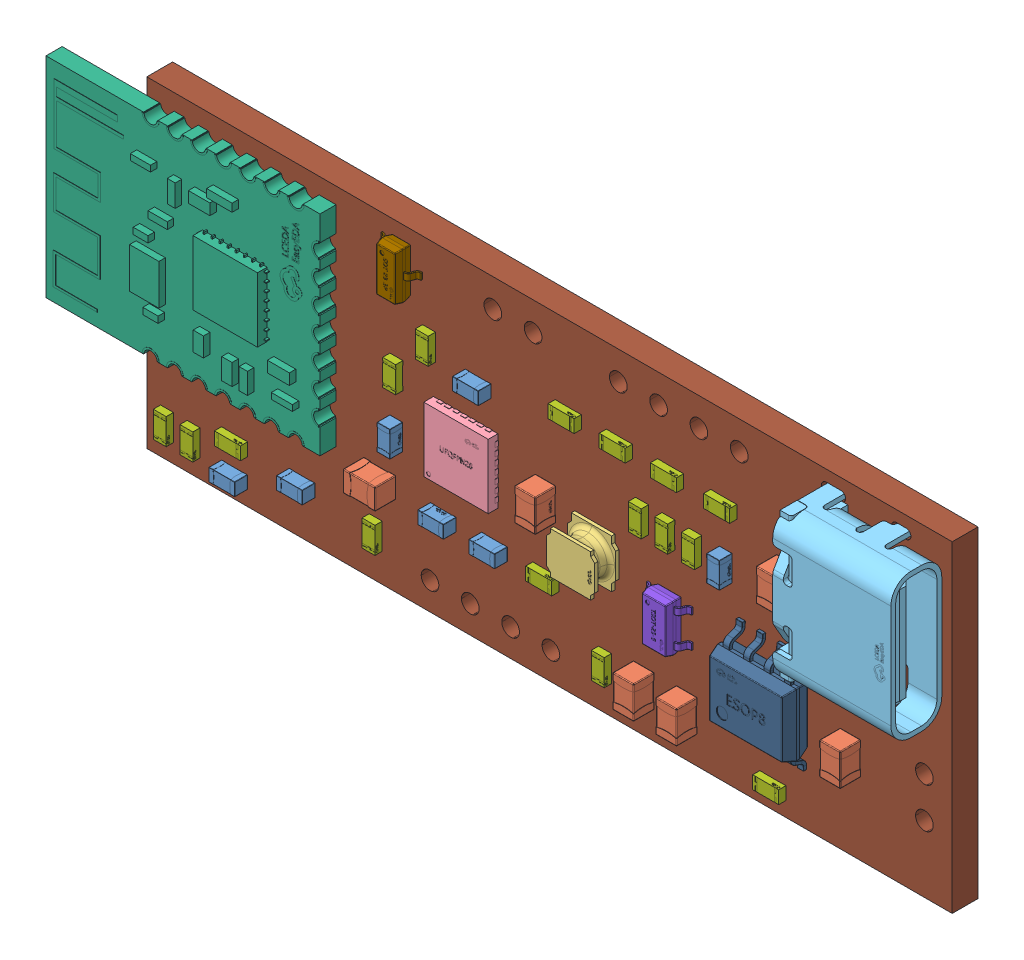
SolidWorks assembly 3D_BOX_2024-11-24, configuration 默认. Lengths in mm.
Overall size (55.21 19.97 4.86).
122 component instances, 13 part files, 0 mates.
Components (placement in the parent):
- 3D_BOX_2024-11-24.step-1: 3D_BOX_2024-11-24.step [默认] at origin size (56.98 23.31 10.6)
  - 3yDE-C2.step-1: 3yDE-C2.step [默认] at (21.082 -14.478 1.6001) x (-1 0 0) z (0 0 1) size (1.6 0.8 0.8)
    - C0603.step-1: C0603.step [默认] at origin size (1.6 0.8 0.8)
      - SOLID.step-1: SOLID.step [默认] at origin size (1.6 0.8 0.8)
  - 3yDE-C3.step-1: 3yDE-C3.step [默认] at (14.986 -11.43 1.6001) x (0 -1 0) z (0 0 1) size (1.6 0.8 0.8)
    - C0603.step-1: C0603.step [默认] at origin size (1.6 0.8 0.8)
      - SOLID.step-1: SOLID.step [默认] at origin size (1.6 0.8 0.8)
  - 3yDE-C4.step-1: 3yDE-C4.step [默认] at (20.066 -6.223 1.6001) x (-1 0 0) z (0 0 1) size (1.6 0.8 0.8)
    - C0603.step-1: C0603.step [默认] at origin size (1.6 0.8 0.8)
      - SOLID.step-1: SOLID.step [默认] at origin size (1.6 0.8 0.8)
  - 3yDE-C5.step-1: 3yDE-C5.step [默认] at (9.144 -17.018 1.6001) x (-1 0 0) z (0 0 1) size (1.6 0.8 0.8)
    - C0603.step-1: C0603.step [默认] at origin size (1.6 0.8 0.8)
      - SOLID.step-1: SOLID.step [默认] at origin size (1.6 0.8 0.8)
  - 3yDE-C6.step-1: 3yDE-C6.step [默认] at (4.953 -18.669 1.6001) x (-1 0 0) z (0 0 1) size (1.6 0.8 0.8)
    - C0603.step-1: C0603.step [默认] at origin size (1.6 0.8 0.8)
      - SOLID.step-1: SOLID.step [默认] at origin size (1.6 0.8 0.8)
  - 3yDE-C11.step-1: 3yDE-C11.step [默认] at (35.4331 -8.255 1.6001) x (0 -1 0) z (0 0 1) size (1.6 0.8 0.8)
    - C0603.step-1: C0603.step [默认] at origin size (1.6 0.8 0.8)
      - SOLID.step-1: SOLID.step [默认] at origin size (1.6 0.8 0.8)
  - 3yDE-C1.step-1: 3yDE-C1.step [默认] at (17.907 -14.478 1.6001) size (1.6 0.8 0.8)
    - C0603.step-1: C0603.step [默认] at origin size (1.6 0.8 0.8)
      - SOLID.step-1: SOLID.step [默认] at origin size (1.6 0.8 0.8)
  - 3yDE-C8.step-1: 3yDE-C8.step [默认] at (24.257 -10.287 1.6001) x (0 -1 0) z (0 0 1) size (2 1.3 1.3)
    - C0805.step-1: C0805.step [默认] at origin size (2 1.3 1.3)
      - SOLID-0.step-1: SOLID-0.step [默认] at origin size (2 1.3 1.3)
  - 3yDE-C9.step-1: 3yDE-C9.step [默认] at (33.0201 -17.272 1.6001) x (0 1 0) z (0 0 1) size (2 1.3 1.3)
    - C0805.step-1: C0805.step [默认] at origin size (2 1.3 1.3)
      - SOLID-0.step-1: SOLID-0.step [默认] at origin size (2 1.3 1.3)
  - 3yDE-C10.step-1: 3yDE-C10.step [默认] at (30.3531 -17.272 1.6001) x (0 1 0) z (0 0 1) size (2 1.3 1.3)
    - C0805.step-1: C0805.step [默认] at origin size (2 1.3 1.3)
      - SOLID-0.step-1: SOLID-0.step [默认] at origin size (2 1.3 1.3)
  - 3yDE-C12.step-1: 3yDE-C12.step [默认] at (39.2431 -7.112 1.6001) x (0 -1 0) z (0 0 1) size (2 1.3 1.3)
    - C0805.step-1: C0805.step [默认] at origin size (2 1.3 1.3)
      - SOLID-0.step-1: SOLID-0.step [默认] at origin size (2 1.3 1.3)
  - 3yDE-C13.step-1: 3yDE-C13.step [默认] at (43.1801 -14.478 1.6001) x (0 1 0) z (0 0 1) size (2 1.3 1.3)
    - C0805.step-1: C0805.step [默认] at origin size (2 1.3 1.3)
      - SOLID-0.step-1: SOLID-0.step [默认] at origin size (2 1.3 1.3)
  - 3yDE-C7.step-1: 3yDE-C7.step [默认] at (13.97 -14.351 1.6001) x (-1 0 0) z (0 0 1) size (2 1.3 1.3)
    - C0805.step-1: C0805.step [默认] at origin size (2 1.3 1.3)
      - SOLID-0.step-1: SOLID-0.step [默认] at origin size (2 1.3 1.3)
  - 3yDE-S1.step-1: 3yDE-S1.step [默认] at (32.5121 -1.778 1.6001) size (12.5 5.7 10)
    - CONN-TH_4P-P2.50_4PIN.step-1: CONN-TH_4P-P2.50_4PIN.step [默认] at origin size (12.5 5.7 10)
      - COMPOUND.step-1: COMPOUND.step [默认] at origin size (12.5 5.7 10) (hidden)
  - 3yDE-DOWNLOAD1.step-1: 3yDE-DOWNLOAD1.step [默认] at (20.828 -18.288 1.6001) x (-1 0 0) z (0 0 1) size (12.5 5.7 10)
    - CONN-TH_4P-P2.50_4PIN.step-1: CONN-TH_4P-P2.50_4PIN.step [默认] at origin size (12.5 5.7 10)
      - COMPOUND.step-1: COMPOUND.step [默认] at origin size (12.5 5.7 10) (hidden)
  - 3yDE-L1.step-1: 3yDE-L1.step [默认] at (27.3051 -11.557 1.6001) x (0 -1 0) z (0 0 1) size (3 3 1.52)
    - IND-SMD_L3.0-W3.0_FNR30XXS.step-1: IND-SMD_L3.0-W3.0_FNR30XXS.step [默认] at origin size (3 3 1.52)
      - SOLID-1.step-1: SOLID-1.step [默认] at origin size (3 3 1.52)
  - 3yDE-U2.step-1: 3yDE-U2.step [默认] at (19.304 -10.287 1.6001) size (4.03 4.03 0.61)
    - UFQFPN-28_L4.0-W4.0-P0.50-BL.step-1: UFQFPN-28_L4.0-W4.0-P0.50-BL.step [默认] at origin size (4.03 4.03 0.61)
      - SOLID-2.step-1: SOLID-2.step [默认] at origin size (4.03 4.03 0.61)
  - 3yDE-BAT1.step-1: 3yDE-BAT1.step [默认] at (47.7521 -14.605 1.6001) x (0 1 0) z (0 0 1) size (7.5 5.9 10.6)
    - CONN-TH_2P-P2.50_HX25003-2A.step-1: CONN-TH_2P-P2.50_HX25003-2A.step [默认] at origin size (7.5 5.9 10.6)
      - COMPOUND-3.step-1: COMPOUND-3.step [默认] at origin size (7.5 5.9 10.6) (hidden)
  - 3yDE-SPOWER1.step-1: 3yDE-SPOWER1.step [默认] at (22.225 -1.778 1.6001) x (-1 0 0) z (0 0 1) size (7.5 5.9 10.6)
    - CONN-TH_2P-P2.50_HX25003-2A.step-1: CONN-TH_2P-P2.50_HX25003-2A.step [默认] at origin size (7.5 5.9 10.6)
      - COMPOUND-3.step-1: COMPOUND-3.step [默认] at origin size (7.5 5.9 10.6) (hidden)
  - 3yDE-USB1.step-1: 3yDE-USB1.step [默认] at (43.9421 -5.334 1.6001) x (0 1 0) z (0 0 1) size (8.95 7.58 4.16)
    - USB-C-SMD_TYPE-C-6PIN-2MD-073.step-1: USB-C-SMD_TYPE-C-6PIN-2MD-073.step [默认] at origin size (8.95 7.58 4.16)
      - COMPOUND-4.step-1: COMPOUND-4.step [默认] at origin size (8.95 7.58 4.16)
  - 3yDE-U1.step-1: 3yDE-U1.step [默认] at (5.969 -7.493 1.6001) x (0 1 0) z (0 0 1) size (13 17 1.62)
    - BULETM-SMD_ZX-D30.step-1: BULETM-SMD_ZX-D30.step [默认] at origin size (13 17 1.62)
      - SOLID-5.step-1: SOLID-5.step [默认] at origin size (13 17 1.62)
  - 3yDE-R2.step-1: 3yDE-R2.step [默认] at (24.2672 -14.4989 1.6001) x (-1 0 0) z (0 0 1) size (1.62 0.81 0.45)
    - R0603.step-1: R0603.step [默认] at origin size (1.62 0.81 0.45)
      - COMPOUND-6.step-1: COMPOUND-6.step [默认] at origin size (1.62 0.81 0.45)
  - 3yDE-R3.step-1: 3yDE-R3.step [默认] at (4.953 -16.891 1.6001) x (-1 0 0) z (0 0 1) size (1.62 0.81 0.45)
    - R0603.step-1: R0603.step [默认] at origin size (1.62 0.81 0.45)
      - COMPOUND-6.step-1: COMPOUND-6.step [默认] at origin size (1.62 0.81 0.45)
  - 3yDE-R4.step-1: 3yDE-R4.step [默认] at (0.762 -18.034 1.6001) x (0 1 0) z (0 0 1) size (1.62 0.81 0.45)
    - R0603.step-1: R0603.step [默认] at origin size (1.62 0.81 0.45)
      - COMPOUND-6.step-1: COMPOUND-6.step [默认] at origin size (1.62 0.81 0.45)
  - 3yDE-R5.step-1: 3yDE-R5.step [默认] at (2.413 -18.034 1.6001) x (0 1 0) z (0 0 1) size (1.62 0.81 0.45)
    - R0603.step-1: R0603.step [默认] at origin size (1.62 0.81 0.45)
      - COMPOUND-6.step-1: COMPOUND-6.step [默认] at origin size (1.62 0.81 0.45)
  - 3yDE-R6.step-1: 3yDE-R6.step [默认] at (13.716 -17.399 1.6001) x (0 1 0) z (0 0 1) size (1.62 0.81 0.45)
    - R0603.step-1: R0603.step [默认] at origin size (1.62 0.81 0.45)
      - COMPOUND-6.step-1: COMPOUND-6.step [默认] at origin size (1.62 0.81 0.45)
  - 3yDE-R7.step-1: 3yDE-R7.step [默认] at (27.9401 -17.399 1.6001) x (0 1 0) z (0 0 1) size (1.62 0.81 0.45)
    - R0603.step-1: R0603.step [默认] at origin size (1.62 0.81 0.45)
      - COMPOUND-6.step-1: COMPOUND-6.step [默认] at origin size (1.62 0.81 0.45)
  - 3yDE-R8.step-1: 3yDE-R8.step [默认] at (35.3061 -5.08 1.6001) x (-1 0 0) z (0 0 1) size (1.62 0.81 0.45)
    - R0603.step-1: R0603.step [默认] at origin size (1.62 0.81 0.45)
      - COMPOUND-6.step-1: COMPOUND-6.step [默认] at origin size (1.62 0.81 0.45)
  - 3yDE-R9.step-1: 3yDE-R9.step [默认] at (32.0041 -5.08 1.6001) x (-1 0 0) z (0 0 1) size (1.62 0.81 0.45)
    - R0603.step-1: R0603.step [默认] at origin size (1.62 0.81 0.45)
      - COMPOUND-6.step-1: COMPOUND-6.step [默认] at origin size (1.62 0.81 0.45)
  - 3yDE-R10.step-1: 3yDE-R10.step [默认] at (28.8291 -5.08 1.6001) x (-1 0 0) z (0 0 1) size (1.62 0.81 0.45)
    - R0603.step-1: R0603.step [默认] at origin size (1.62 0.81 0.45)
      - COMPOUND-6.step-1: COMPOUND-6.step [默认] at origin size (1.62 0.81 0.45)
  - 3yDE-R11.step-1: 3yDE-R11.step [默认] at (25.6541 -5.08 1.6001) x (-1 0 0) z (0 0 1) size (1.62 0.81 0.45)
    - R0603.step-1: R0603.step [默认] at origin size (1.62 0.81 0.45)
      - COMPOUND-6.step-1: COMPOUND-6.step [默认] at origin size (1.62 0.81 0.45)
  - 3yDE-R12.step-1: 3yDE-R12.step [默认] at (30.2261 -8.255 1.6001) x (0 -1 0) z (0 0 1) size (1.62 0.81 0.45)
    - R0603.step-1: R0603.step [默认] at origin size (1.62 0.81 0.45)
      - COMPOUND-6.step-1: COMPOUND-6.step [默认] at origin size (1.62 0.81 0.45)
  - 3yDE-R13.step-1: 3yDE-R13.step [默认] at (31.8771 -8.255 1.6001) x (0 1 0) z (0 0 1) size (1.62 0.81 0.45)
    - R0603.step-1: R0603.step [默认] at origin size (1.62 0.81 0.45)
      - COMPOUND-6.step-1: COMPOUND-6.step [默认] at origin size (1.62 0.81 0.45)
  - 3yDE-R16.step-1: 3yDE-R16.step [默认] at (38.3541 -18.669 1.6001) x (-1 0 0) z (0 0 1) size (1.62 0.81 0.45)
    - R0603.step-1: R0603.step [默认] at origin size (1.62 0.81 0.45)
      - COMPOUND-6.step-1: COMPOUND-6.step [默认] at origin size (1.62 0.81 0.45)
  - 3yDE-R17.step-1: 3yDE-R17.step [默认] at (17.018 -5.588 1.6001) x (0 1 0) z (0 0 1) size (1.62 0.81 0.45)
    - R0603.step-1: R0603.step [默认] at origin size (1.62 0.81 0.45)
      - COMPOUND-6.step-1: COMPOUND-6.step [默认] at origin size (1.62 0.81 0.45)
  - 3yDE-R14.step-1: 3yDE-R14.step [默认] at (33.5281 -8.255 1.6001) x (0 -1 0) z (0 0 1) size (1.62 0.81 0.45)
    - R0603.step-1: R0603.step [默认] at origin size (1.62 0.81 0.45)
      - COMPOUND-6.step-1: COMPOUND-6.step [默认] at origin size (1.62 0.81 0.45)
  - 3yDE-R1.step-1: 3yDE-R1.step [默认] at (14.986 -8.128 1.6001) x (0 -1 0) z (0 0 1) size (1.62 0.81 0.45)
    - R0603.step-1: R0603.step [默认] at origin size (1.62 0.81 0.45)
      - COMPOUND-6.step-1: COMPOUND-6.step [默认] at origin size (1.62 0.81 0.45)
  - 3yDE-U3.step-1: 3yDE-U3.step [默认] at (32.0041 -12.7 1.6001) x (0 -1 0) z (0 0 1) size (2.9 2.81 1.05)
    - TSOT-25_L2.9-W1.6-P0.95-BL.step-1: TSOT-25_L2.9-W1.6-P0.95-BL.step [默认] at origin size (2.9 2.81 1.05)
      - COMPOUND-7.step-1: COMPOUND-7.step [默认] at origin size (2.9 2.81 1.05)
  - 3yDE-Q1.step-1: 3yDE-Q1.step [默认] at (15.367 -2.159 1.6001) x (-1 0 0) z (0 0 1) size (2.5 2.89 1.05)
    - SOT-23-3_L2.9-W1.3-P1.90-LS2.4-BR.step-1: SOT-23-3_L2.9-W1.3-P1.90-LS2.4-BR.step [默认] at origin size (2.5 2.89 1.05)
      - COMPOUND-8.step-1: COMPOUND-8.step [默认] at origin size (2.5 2.89 1.05)
  - 3yDE-U4.step-1: 3yDE-U4.step [默认] at (38.3541 -13.716 1.6001) size (4.9 6.1 1.7)
    - ESOP-8_L4.9-W3.9-P1.27-LS6.0-BL-EP.step-1: ESOP-8_L4.9-W3.9-P1.27-LS6.0-BL-EP.step [默认] at origin size (4.9 6.1 1.7)
      - COMPOUND-9.step-1: COMPOUND-9.step [默认] at origin size (4.9 6.1 1.7)
  - Board.step-1: Board.step [默认] at origin size (49.97 19.97 1.6)
